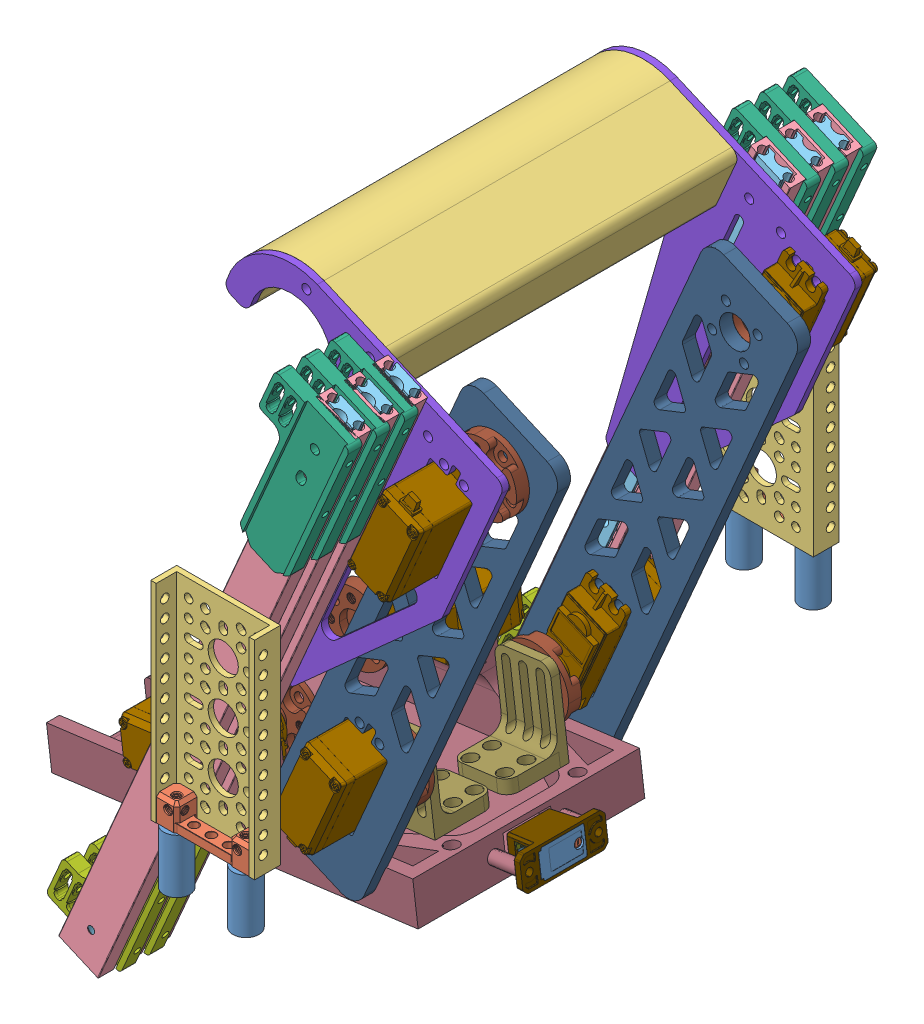
SolidWorks assembly Outtake Sub-Assembly League Meet 3, configuration Default. Lengths in mm.
Overall size (249.3 307.78 277.38).
69 component instances, 21 part files, 63 mates.
Components (placement in the parent):
- 25mm spacer-1: 25mm spacer [Default] at (131.527 64.1625 -130.2749) x (0.98393 0 0.178554) z (-0.178554 0 0.98393) size (12 25 12)
- 25mm spacer-2: 25mm spacer [Default] at (99.527 64.1625 -130.2749) x (0.999949 0 -0.010072) z (0.010072 0 0.999949) size (12 25 12)
- 25mm spacer-4: 25mm spacer [Default] at (131.527 64.1625 132.0751) x (0.974267 0 -0.225397) z (0.225397 0 0.974267) size (12 25 12)
- 25mm spacer-6: 25mm spacer [Default] at (99.527 64.1625 132.0751) x (0.894277 0 -0.447515) z (0.447515 0 0.894277) size (12 25 12)
- dual block.step-1: dual block.step [Default] at (115.527 93.1625 -146.2749) x (0 0 -1) z (0 -1 0) size (9.5 43 12)
- dual block.step-2: dual block.step [Default] at (115.527 93.0375 148.0751) x (0 0 1) z (0 -1 0) size (9.5 43 12)
- 3 Hole Low-Side U Channel 96mm.step-1: 3 Hole Low-Side U Channel 96mm.step [Default] at (94.027 89.0375 148.0751) x (0 0 1) z (-1 0 0) size (12 96 48)
- 3 Hole Low-Side U Channel 96mm.step-2: 3 Hole Low-Side U Channel 96mm.step [Default] at (137.027 89.1625 -146.2749) x (0 0 -1) z (1 0 0) size (12 96 48)
- SAR230 Moveable-1: SAR230 Moveable [Default] at (34.4642 1.8723 -114.1074) x (0 0 1) z (0.396729 0.917936 0) size (8.01 20 300)
  - SAR230_3-1: SAR230_3 [Default] at (5.2 -3.95 0) size (7.4 20 300)
  - SAR230_5-1: SAR230_5 [Default] at (0.0108 0 0) size (5.81 12.1 300)
- LK_Drawer-Slide-Pulley-Insert_v20220723_LH-1: LK_Drawer-Slide-Pulley-Insert_v20220723_LH [Default] at (159.0363 274.8529 -105.7966) x (-0.396729 -0.917936 0) z (0 0 1) size (76.2 37.5 6.35)
- LK_Drawer-Slide-Pulley-Insert_v20220723-1: LK_Drawer-Slide-Pulley-Insert_v20220723 [1_RightHand] at (40.0177 -0.5279 -105.7966) x (0.396729 0.917936 0) z (0 0 1) size (76.2 37.5 6.35)
- LK_Drawer-Slide-Pulley-Insert_v20220723-2: LK_Drawer-Slide-Pulley-Insert_v20220723 [1_RightHand] at (40.0177 -0.5279 -92.7858) x (0.396729 0.917936 0) z (0 0 1) size (76.2 37.5 6.35)
- LK_Drawer-Slide-Pulley-Insert_v20220723_LH-3: LK_Drawer-Slide-Pulley-Insert_v20220723_LH [Default] at (159.0363 274.8529 -92.7858) x (-0.396729 -0.917936 0) z (0 0 1) size (76.2 37.5 6.35)
- SAR230 Moveable-2: SAR230 Moveable [Default] at (34.4642 1.8723 -101.0966) x (0 0 1) z (0.396729 0.917936 0) size (8.01 20 300)
  - SAR230_3-1: SAR230_3 [Default] at (5.2 -3.95 0) size (7.4 20 300)
  - SAR230_5-1: SAR230_5 [Default] at (0.0108 0 0) size (5.81 12.1 300)
- SAR230 Moveable-4: SAR230 Moveable [Default] at (34.4642 1.8723 -88.0858) x (0 0 1) z (0.396729 0.917936 0) size (8.01 20 300)
  - SAR230_3-1: SAR230_3 [Default] at (5.2 -3.95 0) size (7.4 20 300)
  - SAR230_5-1: SAR230_5 [Default] at (0.0108 0 0) size (5.81 12.1 300)
- LK_Drawer-Slide-Pulley-Insert_v20220723_LH-7: LK_Drawer-Slide-Pulley-Insert_v20220723_LH [Default] at (159.0363 274.8529 -118.8074) x (-0.396729 -0.917936 0) z (0 0 1) size (76.2 37.5 6.35)
- SAR230 Moveable-6: SAR230 Moveable [Default] at (45.5712 -2.9281 102.8967) x (0 0 -1) z (0.396729 0.917936 0) size (8.01 20 300)
  - SAR230_3-1: SAR230_3 [Default] at (5.2 -3.95 0) size (7.4 20 300)
  - SAR230_5-1: SAR230_5 [Default] at (0.0108 0 0) size (5.81 12.1 300)
- LK_Drawer-Slide-Pulley-Insert_v20220723_LH-10: LK_Drawer-Slide-Pulley-Insert_v20220723_LH [Default] at (159.0363 274.8529 93.2384) x (-0.396729 -0.917936 0) z (0 0 1) size (76.2 37.5 6.35)
- SAR230 Moveable-7: SAR230 Moveable [Default] at (45.5712 -2.9281 89.8859) x (0 0 -1) z (0.396729 0.917936 0) size (8.01 20 300)
  - SAR230_3-1: SAR230_3 [Default] at (5.2 -3.95 0) size (7.4 20 300)
  - SAR230_5-1: SAR230_5 [Default] at (0.0108 0 0) size (5.81 12.1 300)
- LK_Drawer-Slide-Pulley-Insert_v20220723_LH-11: LK_Drawer-Slide-Pulley-Insert_v20220723_LH [Default] at (159.0363 274.8529 119.2601) x (-0.396729 -0.917936 0) z (0 0 1) size (76.2 37.5 6.35)
- LK_Drawer-Slide-Pulley-Insert_v20220723_LH-12: LK_Drawer-Slide-Pulley-Insert_v20220723_LH [Default] at (159.0363 274.8529 106.2492) x (-0.396729 -0.917936 0) z (0 0 1) size (76.2 37.5 6.35)
- SAR230 Moveable-8: SAR230 Moveable [Default] at (45.5712 -2.9281 115.9076) x (0 0 -1) z (0.396729 0.917936 0) size (8.01 20 300)
  - SAR230_3-1: SAR230_3 [Default] at (5.2 -3.95 0) size (7.4 20 300)
  - SAR230_5-1: SAR230_5 [Default] at (0.0108 0 0) size (5.81 12.1 300)
- LK_Drawer-Slide-Pulley-Insert_v20220723-6: LK_Drawer-Slide-Pulley-Insert_v20220723 [1_RightHand] at (40.0177 -0.5279 106.2467) x (0.396729 0.917936 0) z (0 0 1) size (76.2 37.5 6.35)
- LK_Drawer-Slide-Pulley-Insert_v20220723-7: LK_Drawer-Slide-Pulley-Insert_v20220723 [1_RightHand] at (40.0177 -0.5279 93.2359) x (0.396729 0.917936 0) z (0 0 1) size (76.2 37.5 6.35)
- Servo Mounting Plate Iteration 2-1: Servo Mounting Plate Iteration 2 [Default] at (126.3062 199.1232 -82.2749) x (0.917936 -0.396729 0) z (-0.396729 -0.917936 0) size (125.58 3.17 159)
- Servo Mounting Plate Iteration 2-2: Servo Mounting Plate Iteration 2 [Default] at (126.3062 199.1232 80.9001) x (0.917936 -0.396729 0) z (-0.396729 -0.917936 0) size (125.58 3.17 159)
- servo.step-1: servo.step [Default] at (170.0612 222.7752 69.7001) x (-0.396729 -0.917936 0) z (0 0 -1) size (54.3 20 43.9)
- servo.step-2: servo.step [Default] at (170.0612 222.7752 -67.8999) x (-0.396729 -0.917936 0) z (0 0 1) size (54.3 20 43.9)
- Bar ARm-1: Bar ARm [Default] at (135.883 143.695 59.4001) x (-0.917936 0.396729 0) z (-0.396729 -0.917936 0) size (48 6 240)
- Bar ARm-2: Bar ARm [Default] at (135.883 143.695 -57.5999) x (0.917936 -0.396729 0) z (-0.396729 -0.917936 0) size (48 6 240)
- servo.step-3: servo.step [Default] at (106.4457 75.5842 42.2001) x (0.396729 0.917936 0) z (0 0 -1) size (54.3 20 43.9)
- servo.step-5: servo.step [Default] at (106.4457 75.5842 -40.3999) x (0.396729 0.917936 0) z (0 0 1) size (54.3 20 43.9)
- Assem3^Outtake Sub-Assembly League Meet 3-1: Assem3^Outtake Sub-Assembly League Meet 3 [Default] at origin (virtual)
- 1908-0025-0032.step-3: 1908-0025-0032.step [Default] at (102.538 66.5425 39.9001) x (0.792658 -0.609667 0) z (0.609667 0.792658 0) size (31.98 8 31.98)
- 1908-0025-0032.step-5: 1908-0025-0032.step [Default] at (102.538 66.5425 -38.0999) x (-0.038198 -0.99927 0) z (-0.99927 0.038198 0) size (31.98 8 31.98)
- servo to bay mount-1: servo to bay mount [Default] at (92.9417 39.0698 27.9001) x (0.991593 0.129394 0) z (0 0 1) size (26.07 39 28)
- servo to bay mount-2: servo to bay mount [Default] at (118.7929 42.4432 -26.0999) x (-0.991593 -0.129394 0) z (0 0 -1) size (26.07 39 28)
- 1908-0025-0032.step-6: 1908-0025-0032.step [Default] at (173.969 231.8169 -65.5999) x (1 0 0) z (0 -1 0) size (31.98 8 31.98)
- 1908-0025-0032.step-7: 1908-0025-0032.step [Default] at (173.969 231.8169 67.4001) x (-0.972777 -0.231744 0) z (0.231744 -0.972777 0) size (31.98 8 31.98)
- bay cad-1: bay cad [Default] at (40.3663 26.0998 7.5229) x (0 0 1) z (-0.991593 -0.129394 0) size (146.83 58.11 187.39)
  - bay-1: bay [Default] at (-174.4712 -12.942 -75.9186) size (112.83 54 184.35)
  - servo.step-1: servo.step [Default] at (-41.0779 29.108 0.4679) x (0 0 -1) z (1 0 0) size (54.3 20 43.9)
  - servo.step-2: servo.step [Default] at (29.3521 29.108 0.4679) x (0 0 1) z (-1 0 0) size (54.3 20 43.9)
  - 1908-0025-0032.step-1: 1908-0025-0032.step [Default] at (-38.7779 29.108 10.3179) x (0 -0.99999 -0.004418) z (0 -0.004418 0.99999) size (31.98 8 31.98)
  - 1908-0025-0032.step-2: 1908-0025-0032.step [Default] at (27.0521 29.108 -9.3821) x (0 -0.004418 -0.99999) z (0 0.99999 -0.004418) size (31.98 8 31.98)
  - REV-31-1505.STEP-1: REV-31-1505.STEP [Default] at (-5.8629 -2.832 -108.3821) x (1 0 0) z (0 -1 0) size (39.4 16.64 15)
    - range sensor stacked v1.1.STEP-1: range sensor stacked v1.1.STEP [Default] at (-9.25 12.5 5.5) x (1 0 0) z (0 1 0) size (19.65 11 10.5)
      - range sensor sensor board v1.1.STEP-1: range sensor sensor board v1.1.STEP [Default] at origin size (18.5 11 1.6)
        - range sensor sensor board v1.1-0.STEP-1: range sensor sensor board v1.1-0.STEP [Default] at origin size (18.5 11 1.6)
      - range sensor combined v1.1.STEP-1: range sensor combined v1.1.STEP [Default] at (39.25 0 -5.5) x (-1 0 0) z (0 0 -1) size (19.4 11 8.2)
        - range sensor conector board v1.1.STEP-1: range sensor conector board v1.1.STEP [Default] at origin size (18.5 11 1.6)
        - S4B-PH-K-S.STEP-1: S4B-PH-K-S.STEP [Default] at (30.55 15.25 -6) x (0 1 0) z (-1 0 0) size (9.9 8.2 7.6)
      - REV-41-1532.STEP-1: REV-41-1532.STEP [Default] at (13.55 5.5 -0.7) x (0 -1 0) z (-1 0 0) size (9.9 3.2 6.4)
    - REV-40-1515.STEP-1: REV-40-1515.STEP [Default] at origin size (39.4 16.64 15)
    - REV-40-1516.STEP-1: REV-40-1516.STEP [Default] at origin size (21.1 6.7 12.6)
    - cheese slotted head_ks_KS 1021 CS - M2 x 12-N.STEP-1: cheese slotted head_ks_KS 1021 CS - M2 x 12-N.STEP [Default] at (-7 0.5 0.0007) x (0 1 0) z (0 0 1) size (13.41 3.8 3.8)
- hook connectors-1: hook connectors [Default] at (126.3062 199.1232 -79.0999) x (0.917936 -0.396729 0) z (-0.396729 -0.917936 0) size (66.1 160 38)
Mates (geometry in assembly coordinates):
- Coincident13: coincident anti-aligned: plane of SAR230 Moveable-1/SAR230_5-1 through (153.6663 277.1737 -108.2966) normal (0 0 1); plane of LK_Drawer-Slide-Pulley-Insert_v20220723_LH-1 through (159.0363 274.8529 -108.2966) normal (0 0 -1)
- Coincident14: coincident anti-aligned: plane of SAR230 Moveable-1/SAR230_5-1 through (153.6663 277.1737 -108.2966) normal (0 0 1); plane of LK_Drawer-Slide-Pulley-Insert_v20220723-1 through (40.0177 -0.5279 -108.2966) normal (0 0 -1)
- Concentric13: concentric aligned: circle of SAR230 Moveable-1/SAR230_5-1; cylinder of LK_Drawer-Slide-Pulley-Insert_v20220723-1 through (45.9686 13.2411 -108.2966) axis (0 0 1) radius 2.125
- Parallel3: parallel aligned: plane of SAR230 Moveable-1/SAR230_3-1 through (149.8569 278.8202 -116.0074) normal (-0.917936 0.396729 0); plane of LK_Drawer-Slide-Pulley-Insert_v20220723-1 through (28.5435 4.4312 -103.2966) normal (-0.917936 0.396729 0)
- Concentric14: concentric aligned: circle of SAR230 Moveable-1/SAR230_5-1; cylinder of LK_Drawer-Slide-Pulley-Insert_v20220723_LH-1 through (153.0853 261.0838 -108.2966) axis (0 0 1) radius 2.125
- Parallel4: parallel anti-aligned: plane of SAR230 Moveable-1/SAR230_3-1 through (149.8569 278.8202 -116.0074) normal (-0.917936 0.396729 0); plane of LK_Drawer-Slide-Pulley-Insert_v20220723_LH-1 through (170.5105 269.8938 -103.2966) normal (0.917936 -0.396729 0)
- Coincident17: coincident anti-aligned: plane of LK_Drawer-Slide-Pulley-Insert_v20220723_LH-3 through (159.0363 274.8529 -95.2858) normal (0 0 -1); plane of SAR230 Moveable-2/SAR230_5-1 through (153.6663 277.1737 -95.2858) normal (0 0 1)
- Coincident18: coincident anti-aligned: plane of LK_Drawer-Slide-Pulley-Insert_v20220723-2 through (40.0177 -0.5279 -95.2858) normal (0 0 -1); plane of SAR230 Moveable-2/SAR230_5-1 through (153.6663 277.1737 -95.2858) normal (0 0 1)
- Concentric15: concentric aligned: cylinder of LK_Drawer-Slide-Pulley-Insert_v20220723-2 through (45.9686 13.2411 -95.2858) axis (0 0 1) radius 2.125; circle of SAR230 Moveable-2/SAR230_5-1
- Parallel5: parallel aligned: plane of LK_Drawer-Slide-Pulley-Insert_v20220723-2 through (28.5435 4.4312 -90.2858) normal (-0.917936 0.396729 0); plane of SAR230 Moveable-2/SAR230_3-1 through (149.8569 278.8202 -102.9966) normal (-0.917936 0.396729 0)
- Concentric16: concentric aligned: cylinder of LK_Drawer-Slide-Pulley-Insert_v20220723_LH-3 through (153.0853 261.0838 -95.2858) axis (0 0 1) radius 2.125; circle of SAR230 Moveable-2/SAR230_5-1
- Parallel6: parallel anti-aligned: plane of LK_Drawer-Slide-Pulley-Insert_v20220723_LH-3 through (170.5105 269.8938 -90.2858) normal (0.917936 -0.396729 0); plane of SAR230 Moveable-2/SAR230_3-1 through (149.8569 278.8202 -102.9966) normal (-0.917936 0.396729 0)
- Coincident19: coincident anti-aligned: plane of LK_Drawer-Slide-Pulley-Insert_v20220723_LH-1 through (159.0363 274.8529 -103.2966) normal (0 0 1); plane of SAR230 Moveable-2/SAR230_3-1 through (167.9403 271.0046 -103.2966) normal (0 0 -1)
- Concentric17: concentric aligned: cylinder of SAR230 Moveable-1/SAR230_5-1 through (99.527 137.1625 -108.2966) axis (0 0 1) radius 1.621; cylinder of SAR230 Moveable-2/SAR230_5-1 through (99.527 137.1625 -95.2858) axis (0 0 1) radius 1.621
- Coincident24: coincident anti-aligned: plane of LK_Drawer-Slide-Pulley-Insert_v20220723_LH-3 through (159.0363 274.8529 -90.2858) normal (0 0 1); plane of SAR230 Moveable-4/SAR230_3-1 through (167.9403 271.0046 -90.2858) normal (0 0 -1)
- Concentric22: concentric aligned: cylinder of SAR230 Moveable-2/SAR230_5-1 through (99.527 137.1625 -95.2858) axis (0 0 1) radius 1.621; cylinder of SAR230 Moveable-4/SAR230_5-1 through (99.527 137.1625 -82.2749) axis (0 0 1) radius 1.621
- Coincident27: coincident aligned: plane of SAR230 Moveable-2/SAR230_3-1 through (149.8569 278.8202 -102.9966) normal (-0.917936 0.396729 0); plane of SAR230 Moveable-4/SAR230_3-1 through (149.8569 278.8202 -89.9858) normal (-0.917936 0.396729 0)
- Concentric25: concentric aligned: circle of SAR230 Moveable-1/SAR230_3-1; cylinder of LK_Drawer-Slide-Pulley-Insert_v20220723_LH-7 through (153.0853 261.0838 -121.3074) axis (0 0 1) radius 2.125
- Parallel13: parallel anti-aligned: plane of SAR230 Moveable-1/SAR230_3-1 through (149.8569 278.8202 -116.0074) normal (-0.917936 0.396729 0); plane of LK_Drawer-Slide-Pulley-Insert_v20220723_LH-7 through (170.5105 269.8938 -116.3074) normal (0.917936 -0.396729 0)
- Coincident29: coincident anti-aligned: plane of SAR230 Moveable-1/SAR230_3-1 through (167.9403 271.0046 -116.3074) normal (0 0 -1); plane of LK_Drawer-Slide-Pulley-Insert_v20220723_LH-7 through (159.0363 274.8529 -116.3074) normal (0 0 1)
- Concentric26: concentric aligned: circle of SAR230 Moveable-4/SAR230_5-1; circle of Servo Mounting Plate Iteration 2-1
- Coincident30: coincident anti-aligned: plane of SAR230 Moveable-4/SAR230_5-1 through (153.6663 277.1737 -82.2749) normal (0 0 1); plane of Servo Mounting Plate Iteration 2-1 through (126.3062 199.1232 -82.2749) normal (0 0 -1)
- Concentric27: concentric anti-aligned: circle of SAR230 Moveable-4/SAR230_5-1; cylinder of Servo Mounting Plate Iteration 2-1 through (99.527 137.1625 -79.0999) axis (0 0 -1) radius 2.1
- Coincident113: coincident: plane of dual block.step-1 through (137.027 93.1625 -124.7749) normal (0 0 1); plane of 3 Hole Low-Side U Channel 96mm.step-2 through (137.027 185.1625 -124.7749) normal (0 0 -1)
- Concentric80: concentric: cylinder of 25mm spacer-1 through (131.527 89.1625 -130.2749) axis (0 -1 0) radius 6; circle of dual block.step-1
- Concentric81: concentric: circle of dual block.step-1; cylinder of 3 Hole Low-Side U Channel 96mm.step-2 through (131.527 97.1625 -132.2749) axis (0 0 1) radius 2
- Coincident114: coincident: plane of 25mm spacer-1 through (131.527 89.1625 -130.2749) normal (0 1 0); plane of dual block.step-1 through (115.527 89.1625 -147.5249) normal (0 -1 0)
- Coincident115: coincident: plane of dual block.step-1 through (94.027 93.1625 -124.7749) normal (-1 0 0); plane of 3 Hole Low-Side U Channel 96mm.step-2 through (94.027 79.3391 -134.2749) normal (1 0 0)
- Concentric82: concentric aligned: cylinder of 3 Hole Low-Side U Channel 96mm.step-2 through (99.527 137.1625 -132.2749) axis (0 0 1) radius 2; circle of SAR230 Moveable-1/SAR230_3-1
- Concentric83: concentric: circle of dual block.step-2; cylinder of 3 Hole Low-Side U Channel 96mm.step-1 through (99.527 97.0375 134.0751) axis (0 0 -1) radius 2
- Concentric84: concentric: cylinder of 25mm spacer-4 through (131.527 89.1625 132.0751) axis (0 -1 0) radius 3; circle of dual block.step-2
- Parallel40: parallel: plane of dual block.step-2 through (137.027 93.0375 126.5751) normal (1 0 0); plane of 3 Hole Low-Side U Channel 96mm.step-1 through (139.527 185.0375 126.5751) normal (1 0 0)
- Coincident117: coincident: plane of 25mm spacer-4 through (131.527 89.1625 132.0751) normal (0 1 0); line of dual block.step-2 through (129.027 89.1625 136.0751) axis (1 0 0)
- Coincident118: coincident: plane of dual block.step-2 through (94.027 93.0375 126.5751) normal (0 0 -1); plane of 3 Hole Low-Side U Channel 96mm.step-1 through (94.027 185.0375 126.5751) normal (0 0 1)
- Angle1: planar angle = 0.40795 rad aligned: plane of SAR230 Moveable-2/SAR230_3-1 through (149.8569 278.8202 -102.9966) normal (-0.917936 0.396729 0); plane of 3 Hole Low-Side U Channel 96mm.step-2 through (91.527 185.1625 -124.7749) normal (-1 0 0)
- Coincident144: coincident anti-aligned: plane of 1908-0025-0032.step-3 through (102.538 66.5425 31.9001) normal (0 0 -1); plane of servo to bay mount-1 through (93.5701 73.4401 31.9001) normal (0 0 1)
- Coincident149: coincident anti-aligned: plane of 1908-0025-0032.step-5 through (102.538 66.5425 -30.0999) normal (0 0 1); plane of servo to bay mount-2 through (109.3658 75.5013 -30.0999) normal (0 0 -1)
- Parallel48: parallel aligned: plane of SAR230 Moveable-7/SAR230_3-1 through (168.2156 270.8856 91.7859) normal (0.917936 -0.396729 0); plane of Bar ARm-1 through (110.306 24.0212 53.4001) normal (0.917936 -0.396729 0)
- Concentric128: concentric anti-aligned: circle of 1908-0025-0032.step-3; cylinder of servo to bay mount-1 through (93.5701 73.4401 31.9001) axis (0 0 -1) radius 2
- Concentric129: concentric anti-aligned: circle of 1908-0025-0032.step-3; cylinder of servo to bay mount-1 through (109.4355 75.5104 31.9001) axis (0 0 -1) radius 2
- Concentric131: concentric anti-aligned: circle of servo.step-1; cylinder of Bar ARm-1 through (173.969 231.8169 53.4001) axis (0 0 1) radius 7.1
- Coincident151: coincident anti-aligned: plane of Servo Mounting Plate Iteration 2-2 through (126.3062 199.1232 80.9001) normal (0 0 -1); plane of servo.step-1 through (152.0826 202.6023 80.9001) normal (0 0 1)
- Concentric132: concentric aligned: cylinder of Servo Mounting Plate Iteration 2-2 through (165.0835 198.7809 84.0751) axis (0 0 -1) radius 2.1; cylinder of servo.step-1 through (165.0835 198.7809 80.9011) axis (0 0 -1) radius 2.25
- Parallel49: parallel aligned: plane of Servo Mounting Plate Iteration 2-2 through (203.2664 252.4686 84.0751) normal (0.917936 -0.396729 0); plane of servo.step-1 through (169.0644 195.2629 78.2001) normal (0.917936 -0.396729 0)
- Concentric133: concentric anti-aligned: cylinder of Bar ARm-1 through (120.511 95.6508 53.4001) axis (0 0 1) radius 2.1; cylinder of servo.step-3 through (120.511 95.6508 53.4011) axis (0 0 -1) radius 2.25
- Parallel50: parallel aligned: plane of Bar ARm-1 through (110.306 24.0212 53.4001) normal (0.917936 -0.396729 0); plane of servo.step-3 through (123.3415 89.4707 53.4001) normal (0.917936 -0.396729 0)
- Coincident155: coincident anti-aligned: plane of servo.step-3 through (102.538 66.5425 36.5001) normal (0 0 -1); plane of 1908-0025-0032.step-3 through (102.538 66.5425 36.5001) normal (0 0 1)
- Coincident156: coincident anti-aligned: plane of Bar ARm-1 through (135.883 143.695 53.4001) normal (0 0 -1); plane of servo.step-3 through (124.4243 95.757 53.4001) normal (0 0 1)
- Concentric134: concentric anti-aligned: cylinder of Bar ARm-1 through (173.969 231.8169 53.4001) axis (0 0 1) radius 7.1; cylinder of 1908-0025-0032.step-6 through (173.969 231.8169 -57.5999) axis (0 0 -1) radius 15.99
- Concentric135: concentric aligned: cylinder of Bar ARm-1 through (173.969 231.8169 53.4001) axis (0 0 1) radius 7.1; cylinder of 1908-0025-0032.step-7 through (173.969 231.8169 59.4001) axis (0 0 1) radius 15.99
- Coincident160: coincident anti-aligned: plane of servo.step-1 through (173.969 231.8169 64.0001) normal (0 0 -1); plane of 1908-0025-0032.step-7 through (173.969 231.8169 64.0001) normal (0 0 1)
- Coincident161: coincident anti-aligned: plane of Bar ARm-1 through (135.883 143.695 59.4001) normal (0 0 1); plane of 1908-0025-0032.step-7 through (173.969 231.8169 59.4001) normal (0 0 -1)
- Coincident162: coincident aligned: plane of servo to bay mount-1 through (118.0166 48.3928 27.9001) normal (0.991593 0.129394 0); plane of servo to bay mount-2 through (118.0166 48.3928 -7.0999) normal (0.991593 0.129394 0)
- Concentric139: concentric aligned: cylinder of servo.step-3 through (102.538 66.5425 40.5001) axis (0 0 1) radius 5.45; cylinder of 1908-0025-0032.step-3 through (102.538 66.5425 -13.3265) axis (0 0 1) radius 4.99
- Coincident166: coincident anti-aligned: plane of servo.step-5 through (102.538 66.5425 -34.6999) normal (0 0 1); plane of 1908-0025-0032.step-5 through (102.538 66.5425 -34.6999) normal (0 0 -1)
- Concentric141: concentric aligned: circle of servo.step-5; cylinder of 1908-0025-0032.step-5 through (102.538 66.5425 15.1266) axis (0 0 -1) radius 4.99
- Coincident175: coincident anti-aligned: plane of servo to bay mount-1 through (113.835 41.7962 8.9001) normal (0.129394 -0.991593 0); plane of bay cad-1/bay-1 through (114.8628 41.9304 -166.9483) normal (-0.129394 0.991593 0)
- Coincident176: coincident aligned: plane of servo to bay mount-1 through (113.0586 47.7458 8.9001) normal (-0.129394 0.991593 0); plane of servo to bay mount-2 through (97.1233 45.6664 -7.0999) normal (-0.129394 0.991593 0)
- Distance2: distance = 30 mm anti-aligned: plane of bay cad-1/bay-1 through (116.8684 26.5607 54.0751) normal (0 0 1); plane of SAR230 Moveable-7/SAR230_5-1 through (164.4062 272.532 84.0751) normal (0 0 -1)
- Distance3: distance = 12 mm aligned: plane of servo to bay mount-1 through (118.0166 48.3928 27.9001) normal (0.991593 0.129394 0); plane of bay cad-1/bay-1 through (132.6977 28.6262 -166.9483) normal (0.991593 0.129394 0)
- Coincident180: coincident anti-aligned: plane of Servo Mounting Plate Iteration 2-2 through (126.3062 199.1232 80.9001) normal (0 0 -1); plane of hook connectors-1 through (104.1746 261.4698 80.9001) normal (0 0 1)
- Concentric148: concentric anti-aligned: circle of Servo Mounting Plate Iteration 2-1; cylinder of hook connectors-1 through (111.4832 285.6005 -74.3999) axis (0 0 -1) radius 3.1
- Concentric149: concentric anti-aligned: cylinder of Servo Mounting Plate Iteration 2-1 through (140.8572 272.9052 -82.2749) axis (0 0 1) radius 2.1; cylinder of hook connectors-1 through (140.8572 272.9052 -74.3999) axis (0 0 -1) radius 3.1
